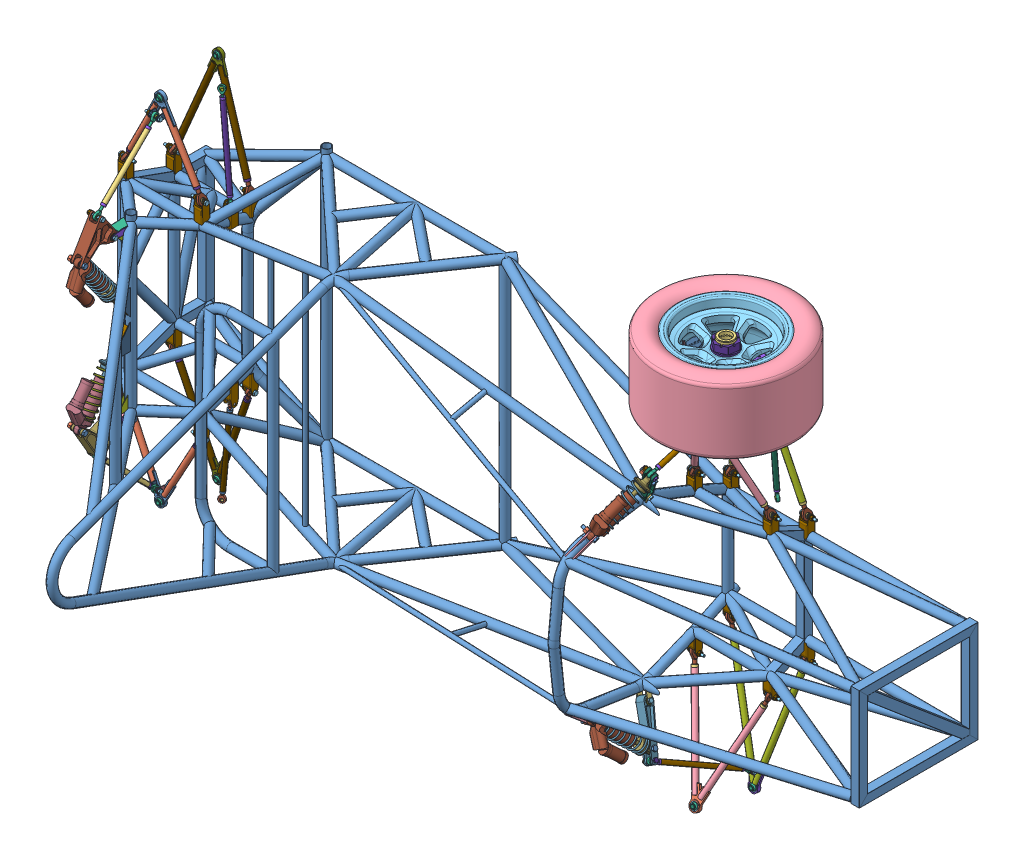
SolidWorks assembly AE-Rolling Chassis Assembly, configuration Default. Lengths in mm. (continued)
Components (placement in the parent): (continued)
- SP-A0200-AI-Rear Axle Assembly-1: SP-A0200-AI-Rear Axle Assembly [Default] at (222.4405 0 -72.1526) size (274.88 1137.82 484.64)
  - SP-AA-Rear Lower A-Arm^SP-A0200-AI-Rear Axle Assembly-1: SP-AA-Rear Lower A-Arm^SP-A0200-AI-Rear Axle Assembly [Default] at (0 -0.399 0.6588) x (1 0 0) z (0 0.002866 0.999996) size (222.76 290.57 36.42) (virtual)
    - SP-Lower Apex Rear-1: SP-Lower Apex Rear [Default] at (-792.4265 549.6462 121.5417) x (-0.932505 -0.360479 0.022123) z (0 -0.061256 -0.998122) size (54.94 63.8 9.53)
    - SP-10003-AB-Threaded Insert-1: SP-10003-AB-Threaded Insert [A-Arm] at (-890.6731 296.4508 137.0806) x (0.932505 -0.360479 0.022123) z (-0.361157 -0.930754 0.057121) size (15.88 15.88 15.88)
    - SP-10003-AB-Threaded Insert-2: SP-10003-AB-Threaded Insert [A-Arm] at (-694.18 296.4508 137.0806) x (0.932505 0.360479 -0.022123) z (0.361157 -0.930754 0.057121) size (15.88 15.88 15.88)
    - SP-Rear Lower A-Arm Tube-1: SP-Rear Lower A-Arm Tube [Default] at (-838.6322 430.5677 128.8497) x (-0.361157 -0.930754 0.057121) z (0 -0.061256 -0.998122) size (257.84 15.88 15.88)
    - SP-Rear Lower A-Arm Tube-2: SP-Rear Lower A-Arm Tube [Default] at (-746.2209 430.5677 128.8497) x (0.361157 -0.930754 0.057121) z (0 0.061256 0.998122) size (257.84 15.88 15.88)
    - FS-HIGH MISALIGN SPHERICAL BEARING, 0.375-0.906D (3072-6G)-1: FS-HIGH MISALIGN SPHERICAL BEARING, 0.375-0.906D (3072-6G) [Default] at (-792.4265 549.6462 121.5417) x (-0.932505 0.360479 -0.022123) z (-0.361157 -0.930754 0.057121) size (26.46 21.71 26.13)
      - Race^FS-HIGH MISALIGN SPHERICAL BEARING, 0.375-0.906D (3072-6G)-1: Race^FS-HIGH MISALIGN SPHERICAL BEARING, 0.375-0.906D (3072-6G) [Default] at origin size (23.01 8.76 23.01) (virtual)
      - Ball^FS-HIGH MISALIGN SPHERICAL BEARING, 0.375-0.906D (3072-6G)-1: Ball^FS-HIGH MISALIGN SPHERICAL BEARING, 0.375-0.906D (3072-6G) [Default] x (0.359576 -0.008176 0.93308) z (-0.932238 -0.046516 0.358844) size (19.84 20.65 19.84) (virtual)
  - SP-AA-Rear Upper A-Arm^SP-A0200-AI-Rear Axle Assembly-1: SP-AA-Rear Upper A-Arm^SP-A0200-AI-Rear Axle Assembly [Default] at (-38.1 -1.9308 1.9372) x (1 0 0) z (0 0.00685 0.999977) size (216 215.55 29.43) (virtual)
    - SP-Upper Apex Rear-1: SP-Upper Apex Rear [Default] at (-755.8405 523.8827 293.8505) x (0.884705 -0.465567 -0.023329) z (0 -0.050046 0.998747) size (76.45 83.12 9.53)
    - SP-10003-AB-Threaded Insert-1: SP-10003-AB-Threaded Insert [A-Arm] at (-849.4201 346.5014 284.9623) x (0.884705 -0.465567 -0.023329) z (-0.466151 -0.883596 -0.044276) size (15.88 15.88 15.88)
    - SP-10003-AB-Threaded Insert-2: SP-10003-AB-Threaded Insert [A-Arm] at (-662.261 346.5014 284.9623) x (0.884705 0.465567 0.023329) z (0.466151 -0.883596 -0.044276) size (15.88 15.88 15.88)
    - SP-Rear Upper A-Arm Tube-1: SP-Rear Upper A-Arm Tube [Default] at (-812.9905 415.5541 288.4224) x (0.466151 0.883596 0.044276) z (0.884705 -0.465567 -0.023329) size (186.28 15.88 15.88)
    - SP-Rear Upper A-Arm Tube-2: SP-Rear Upper A-Arm Tube [Default] at (-698.6905 415.5541 288.4224) x (-0.466151 0.883596 0.044276) z (0.884705 0.465567 0.023329) size (186.28 15.88 15.88)
    - FS-HIGH MISALIGN SPHERICAL BEARING, 0.375-0.906D (3072-6G)-1: FS-HIGH MISALIGN SPHERICAL BEARING, 0.375-0.906D (3072-6G) [Default] at (-755.8405 523.8827 293.8505) x (0.884705 -0.465567 -0.023329) z (-0.466151 -0.883596 -0.044276) size (26.46 21.71 26.13)
      - Race^FS-HIGH MISALIGN SPHERICAL BEARING, 0.375-0.906D (3072-6G)-1: Race^FS-HIGH MISALIGN SPHERICAL BEARING, 0.375-0.906D (3072-6G) [Default] at origin size (23.01 8.76 23.01) (virtual)
      - Ball^FS-HIGH MISALIGN SPHERICAL BEARING, 0.375-0.906D (3072-6G)-1: Ball^FS-HIGH MISALIGN SPHERICAL BEARING, 0.375-0.906D (3072-6G) [Default] x (0.359576 -0.008176 0.93308) z (-0.932238 -0.046516 0.358844) size (19.84 20.65 19.84) (virtual)
  - Assem8^SP-A0200-AI-Rear Axle Assembly-1: Assem8^SP-A0200-AI-Rear Axle Assembly [Default] at (-1592.9214 814.7933 712.2762) x (-0.999891 -0.01037 0.010464) z (0.012143 -0.982316 0.186836) size (17.98 166.51 230.13) (virtual)
    - Part2^Assem8_SP-A0200-AI-Rear Axle Assembly-1: Part2^Assem8_SP-A0200-AI-Rear Axle Assembly [Default] at origin size (15.39 113.92 157.78) (virtual)
    - SP-10003-AC-Threaded Insert-2: SP-10003-AC-Threaded Insert [AM-4 Rod End Thread] at (-799.064 427.6015 294.0449) x (-0.999891 -0.008342 0.012143) z (-0.014733 0.566176 -0.824153) size (12.7 12.7 15.88)
    - SP-10003-AC-Threaded Insert-3: SP-10003-AC-Threaded Insert [AM-4 Rod End Thread] at (-796.6527 334.9355 428.9338) x (-0.999891 -0.008342 0.012143) z (0.014733 -0.566176 0.824153) size (12.7 12.7 15.88)
    - FS-MALE ROD END UNF-3A, 0.25x28-0.25D (AM-4)-1: FS-MALE ROD END UNF-3A, 0.25x28-0.25D (AM-4) [Default] at (-796.0446 311.5665 462.9507) x (0 -0.824242 -0.566238) z (-0.014733 0.566176 -0.824153) size (19.32 14.06 49.44)
      - Body^FS-MALE ROD END UNF-3A, 0.25x28-0.25D (AM-4)-2: Body^FS-MALE ROD END UNF-3A, 0.25x28-0.25D (AM-4) [Default] at origin size (19.32 7.2 49.44) (virtual)
      - Ball^FS-MALE ROD END UNF-3A, 0.25x28-0.25D (AM-4)-2: Ball^FS-MALE ROD END UNF-3A, 0.25x28-0.25D (AM-4) [Default] x (0.09633 0.218783 0.971007) z (-0.984027 0.167661 0.059845) size (12.7 9.53 12.7) (virtual)
    - FS-MALE ROD END UNF-3A, 0.25x28-0.25D (AM-4)-2: FS-MALE ROD END UNF-3A, 0.25x28-0.25D (AM-4) [Default] at (-799.6721 450.9704 260.028) x (0 -0.824242 -0.566238) z (0.014733 -0.566176 0.824153) size (19.32 14.06 49.44)
      - Body^FS-MALE ROD END UNF-3A, 0.25x28-0.25D (AM-4)-2: Body^FS-MALE ROD END UNF-3A, 0.25x28-0.25D (AM-4) [Default] at origin size (19.32 7.2 49.44) (virtual)
      - Ball^FS-MALE ROD END UNF-3A, 0.25x28-0.25D (AM-4)-2: Ball^FS-MALE ROD END UNF-3A, 0.25x28-0.25D (AM-4) [Default] x (0.09633 0.218783 0.971007) z (-0.984027 0.167661 0.059845) size (12.7 9.53 12.7) (virtual)
  - SP-A0105-AC-Ohlin TTX25 MKII, 200mm-1: SP-A0105-AC-Ohlin TTX25 MKII, 200mm [Default] at (-793.9406 216.4917 537.8809) x (-1 0 0) z (0 0.803503 0.5953) size (48.39 85.02 197.6)
    - Shock Body^SP-A0105-AC-Ohlin TTX25 MKII, 200mm-1: Shock Body^SP-A0105-AC-Ohlin TTX25 MKII, 200mm [Default] at origin size (40.76 80 131.7) (virtual)
    - Head^SP-A0105-AC-Ohlin TTX25 MKII, 200mm-1: Head^SP-A0105-AC-Ohlin TTX25 MKII, 200mm [Default] at (0 0 -174.6) size (46 46 119) (virtual)
    - Ball^SP-A0105-AC-Ohlin TTX25 MKII, 200mm-1: Ball^SP-A0105-AC-Ohlin TTX25 MKII, 200mm [Default] at (0 0 -174.6) x (-0.011681 0.107343 0.994153) z (0.993776 0.111394 -0.000351) size (15 15 8) (virtual)
    - Ball^SP-A0105-AC-Ohlin TTX25 MKII, 200mm-2: Ball^SP-A0105-AC-Ohlin TTX25 MKII, 200mm [Default] x (0.079523 -0.862756 -0.499328) z (0.965926 -0.057074 0.252448) size (15 15 8) (virtual)
    - SP-#####-AB-Spring-1: SP-#####-AB-Spring [Default] at (0 0 -151.1) size (48.39 49.05 127.97)
  - FS-BALL BEARING, 0.25ID-0.75OD (60355K702)-1: FS-BALL BEARING, 0.25ID-0.75OD (60355K702) [Default] at (-784.8125 243.84 446.6415) x (0 -0.287121 0.957894) z (-1 0 0) size (19.05 19.05 7.14)
  - FS-BALL BEARING, 0.25ID-0.75OD (60355K702)-2: FS-BALL BEARING, 0.25ID-0.75OD (60355K702) [Default] at (-803.0688 243.84 446.6415) x (0 0.287121 -0.957894) z (1 0 0) size (19.05 19.05 7.14)
  - FS-CADMIUM PLATED C3 HEX, 0.25x28-1.65-0.469 (AN4-13A)-2: FS-CADMIUM PLATED C3 HEX, 0.25x28-1.65-0.469 (AN4-13A) [Default] at (-796.8362 310.0391 484.3789) x (-1 0 0) z (0 0.868755 0.495242) size (46.28 12.9 11.18)
  - FS-ZINC YELLOW CHROMATE C10.9 HX, M8x1.25-40-22 (95327A569)-1: FS-ZINC YELLOW CHROMATE C10.9 HX, M8x1.25-40-22 (95327A569) [Default] at (-795.4156 216.4917 537.8809) x (-1 0 0) z (0 -0.287121 0.957894) size (45.3 15.01 13)
  - FS-NYLOC FLHX C8, M8x1.25-11.1 (92461A400)-1: FS-NYLOC FLHX C8, M8x1.25-11.1 (92461A400) [Default] at (-820.9156 216.4917 537.8809) x (0 0.868058 -0.496463) z (-1 0 0) size (17.9 17.9 11.1)
  - FS-NYLOC G8 HX, 0.25x28-0.3125 (90630A145)-1: FS-NYLOC G8 HX, 0.25x28-0.3125 (90630A145) [Default] at (-809.8156 310.0391 484.3789) x (0 0.868058 -0.496463) z (0 0.496463 0.868058) size (11.11 7.94 12.83)
  - SP-C30066-AA-A-Arm Tab Box-1: SP-C30066-AA-A-Arm Tab Box [Default] at (-680.9758 289.7175 282.8202) x (-0.029021 0.999579 0) z (0 0 -1) size (60.32 25.4 25.4)
  - SP-C30066-AA-A-Arm Tab Box-2: SP-C30066-AA-A-Arm Tab Box [Default] at (-908.2405 289.7636 282.8202) x (0 1 0) z (0 0 -1) size (60.32 25.4 25.4)
  - SP-C30066-AA-A-Arm Tab Box-3: SP-C30066-AA-A-Arm Tab Box [Default] at (-678.1265 237.6164 139.5469) x (0 1 0) z (0 0 1) size (60.32 25.4 25.4)
  - SP-C30066-AA-A-Arm Tab Box-4: SP-C30066-AA-A-Arm Tab Box [Default] at (-906.7265 237.6164 139.5469) x (0 1 0) z (0 0 1) size (60.32 25.4 25.4)
  - SP-30063-AB- Front Pushrod Tab-1: SP-30063-AB- Front Pushrod Tab [Default] at (-782.0343 483.2134 293.6084) x (1 0 0) z (0 0.043203 -0.999066) size (1.59 15.88 23.81)
  - SP-30063-AB- Front Pushrod Tab-2: SP-30063-AB- Front Pushrod Tab [Default] at (-805.8468 483.2134 293.6084) x (-1 0 0) z (0 0.043203 -0.999066) size (1.59 15.88 23.81)
  - FS-NYLOC FLHX C8, M8x1.25-11.1 (92461A400)-2: FS-NYLOC FLHX C8, M8x1.25-11.1 (92461A400) [Default] at (-820.9156 243.84 446.6415) x (0 0 -1) z (-1 0 0) size (17.9 17.9 11.1)
  - FS-CADMIUM PLATED C3 HEX, 0.25x28-1.65-0.469 (AN4-13A)-3: FS-CADMIUM PLATED C3 HEX, 0.25x28-1.65-0.469 (AN4-13A) [Default] at (-796.8362 243.84 446.6415) x (-1 0 0) z (0 0.287121 -0.957894) size (46.28 12.9 11.18)
  - FS-CADMIUM PLATED C3 HEX, 0.25x28-1.65-0.469 (AN4-13A)-4: FS-CADMIUM PLATED C3 HEX, 0.25x28-1.65-0.469 (AN4-13A) [Default] at (-687.5506 306.9965 282.8202) x (-0.999579 -0.029021 0) z (0 0 -1) size (46.28 12.9 11.18)
  - FS-CADMIUM PLATED C3 HEX, 0.25x28-1.65-0.469 (AN4-13A)-5: FS-CADMIUM PLATED C3 HEX, 0.25x28-1.65-0.469 (AN4-13A) [Default] at (-902.1699 307.2261 282.8202) size (46.28 12.9 11.18)
  - FS-CADMIUM PLATED C3 HEX, 0.25x28-1.65-0.469 (AN4-13A)-6: FS-CADMIUM PLATED C3 HEX, 0.25x28-1.65-0.469 (AN4-13A) [Default] at (-912.7971 255.0789 139.5469) x (-1 0 0) z (0 0 -1) size (46.28 12.9 11.18)
  - FS-CADMIUM PLATED C3 HEX, 0.25x28-1.65-0.469 (AN4-13A)-7: FS-CADMIUM PLATED C3 HEX, 0.25x28-1.65-0.469 (AN4-13A) [Default] at (-684.1971 255.0789 139.5469) x (-1 0 0) z (0 0 -1) size (46.28 12.9 11.18)
  - FS-CADMIUM PLATED C3 HEX, 0.25x28-1.65-0.469 (AN4-13A)-8: FS-CADMIUM PLATED C3 HEX, 0.25x28-1.65-0.469 (AN4-13A) [Default] at (-799.2174 482.5275 309.4686) x (-1 0 0) z (0 -0.609051 0.793131) size (46.28 12.9 11.18)
  - FS-NYLOC G8 HX, 0.25x28-0.3125 (90630A145)-3: FS-NYLOC G8 HX, 0.25x28-0.3125 (90630A145) [Default] at (-807.4343 482.5275 309.4686) x (0 -0.043203 0.999066) z (0 -0.999066 -0.043203) size (11.11 7.94 12.83)
  - FS-NYLOC G8 HX, 0.25x28-0.3125 (90630A145)-4: FS-NYLOC G8 HX, 0.25x28-0.3125 (90630A145) [Default] at (-694.1772 306.8041 282.8202) x (-0.029021 0.999579 0) z (0 0 1) size (11.11 7.94 12.83)
  - FS-NYLOC G8 HX, 0.25x28-0.3125 (90630A145)-5: FS-NYLOC G8 HX, 0.25x28-0.3125 (90630A145) [Default] at (-895.5405 307.2261 282.8202) x (0 1 0) z (0 0 -1) size (11.11 7.94 12.83)
  - FS-NYLOC G8 HX, 0.25x28-0.3125 (90630A145)-6: FS-NYLOC G8 HX, 0.25x28-0.3125 (90630A145) [Default] at (-919.4265 255.0789 139.5469) x (0 1 0) z (0 0 1) size (11.11 7.94 12.83)
  - FS-NYLOC G8 HX, 0.25x28-0.3125 (90630A145)-7: FS-NYLOC G8 HX, 0.25x28-0.3125 (90630A145) [Default] at (-690.8265 255.0789 139.5469) x (0 -1 0) z (0 0 -1) size (11.11 7.94 12.83)
  - FS-ROD END RETAINING WASHER, 0.25-0.245 (NO PN)-5: FS-ROD END RETAINING WASHER, 0.25-0.245 (NO PN) [Default] at (-781.9073 482.5275 309.4686) x (0 1 0) z (-1 0 0) size (12.7 12.7 6.22)
  - FS-ROD END RETAINING WASHER, 0.25-0.245 (NO PN)-6: FS-ROD END RETAINING WASHER, 0.25-0.245 (NO PN) [Default] at (-805.9738 482.5275 309.4686) x (0 0.978954 0.204082) z (1 0 0) size (12.7 12.7 6.22)
  - SP-A0200-Rear Inner Rocker Gusset-1: SP-A0200-Rear Inner Rocker Gusset [Default] at (-793.9406 234.6955 425.4808) x (1 0 0) z (0 0.052336 0.99863) size (26.99 1.59 48.67)
  - SP-A0200-Rear Long Rocker Tab-1: SP-A0200-Rear Long Rocker Tab [Rear] at (-807.4344 243.84 446.6415) x (1 0 0) z (0 -0.00621 -0.999981) size (1.59 19.05 73.11)
  - SP-A0200-Rear Outer Rocker Gusset-1: SP-A0200-Rear Outer Rocker Gusset [Default] at (-793.9406 251.3902 418.9606) x (1 0 0) z (0 -0.039929 0.999203) size (26.99 1.59 43.52)
  - SP-A0200-Rear Rocker Gusset Support-1: SP-A0200-Rear Rocker Gusset Support [Default] at (-800.2906 228.5949 403.7833) x (0 0 1) z (0 1 0) size (38.05 1.59 40.09)
  - SP-A0200-Rear Short Rocker Tab-1: SP-A0200-Rear Short Rocker Tab [Rear] at (-780.4469 243.8408 446.6212) x (1 0 0) z (0 -0.00621 -0.999981) size (1.59 17.17 50.59)
  - SP-A0200-Rear Rocker Gusset Support-2: SP-A0200-Rear Rocker Gusset Support [Default] at (-789.8131 228.5949 403.7833) x (0 0 1) z (0 1 0) size (38.05 1.59 40.09)
  - SP-A0200-Rear Shock Gusset-1: SP-A0200-Rear Shock Gusset [Default] at (-793.9406 34.3591 413.4634) x (1 0 0) z (0 0.809017 0.587785) size (14.29 1.59 50.8)
  - SP-A0200-Rear Shock Tab-1: SP-A0200-Rear Shock Tab [Rear] at (-786.7969 76.2 433.9415) x (-1 0 0) z (0 -0.809017 -0.587785) size (1.59 45.95 88.76)
  - SP-A0200-Rear Shock Tab-2: SP-A0200-Rear Shock Tab [Front] at (-801.0844 76.2 433.9415) x (-1 0 0) z (0 -0.809017 -0.587785) size (1.59 45.95 88.76)
  - FS-MALE ROD END UNJF-3A, 0.375x24-0.25D (HXAM-4T)-4: FS-MALE ROD END UNJF-3A, 0.375x24-0.25D (HXAM-4T) [Simplified] at (-679.6405 307.2261 282.8202) x (0 0.043203 -0.999066) z (-0.466151 0.883879 0.038222) size (26.22 15.06 62.54)
    - Body^FS-MALE ROD END UNJF-3A, 0.375x24-0.25D (HXAM-4T)-1: Body^FS-MALE ROD END UNJF-3A, 0.375x24-0.25D (HXAM-4T) [no_threads] at origin size (26.22 9.62 62.54)
    - Ball^FS-MALE ROD END UNJF-3A, 0.375x24-0.25D (HXAM-4T)-1: Ball^FS-MALE ROD END UNJF-3A, 0.375x24-0.25D (HXAM-4T) [Default] at origin size (15.06 15.06 15.06)
  - FS-MALE ROD END UNJF-3A, 0.375x24-0.25D (HXAM-4T)-5: FS-MALE ROD END UNJF-3A, 0.375x24-0.25D (HXAM-4T) [Simplified] at (-908.2405 307.2261 282.8202) x (0 -0.043203 0.999066) z (0.466151 0.883879 0.038222) size (26.22 15.06 62.54)
    - Body^FS-MALE ROD END UNJF-3A, 0.375x24-0.25D (HXAM-4T)-1: Body^FS-MALE ROD END UNJF-3A, 0.375x24-0.25D (HXAM-4T) [no_threads] at origin size (26.22 9.62 62.54)
    - Ball^FS-MALE ROD END UNJF-3A, 0.375x24-0.25D (HXAM-4T)-1: Ball^FS-MALE ROD END UNJF-3A, 0.375x24-0.25D (HXAM-4T) [Default] at origin size (15.06 15.06 15.06)
  - FS-MALE ROD END UNJF-3A, 0.375x24-0.25D (HXAM-4T)-6: FS-MALE ROD END UNJF-3A, 0.375x24-0.25D (HXAM-4T) [Simplified] at (-906.7265 255.0789 139.5469) x (0 0.064116 0.997942) z (0.361157 0.930586 -0.059789) size (26.22 15.06 62.54)
    - Body^FS-MALE ROD END UNJF-3A, 0.375x24-0.25D (HXAM-4T)-1: Body^FS-MALE ROD END UNJF-3A, 0.375x24-0.25D (HXAM-4T) [no_threads] at origin size (26.22 9.62 62.54)
    - Ball^FS-MALE ROD END UNJF-3A, 0.375x24-0.25D (HXAM-4T)-1: Ball^FS-MALE ROD END UNJF-3A, 0.375x24-0.25D (HXAM-4T) [Default] at origin size (15.06 15.06 15.06)
  - FS-MALE ROD END UNJF-3A, 0.375x24-0.25D (HXAM-4T)-7: FS-MALE ROD END UNJF-3A, 0.375x24-0.25D (HXAM-4T) [Simplified] at (-678.1265 255.0789 139.5469) x (0 -0.064116 -0.997942) z (-0.361157 0.930586 -0.059789) size (26.22 15.06 62.54)
    - Body^FS-MALE ROD END UNJF-3A, 0.375x24-0.25D (HXAM-4T)-1: Body^FS-MALE ROD END UNJF-3A, 0.375x24-0.25D (HXAM-4T) [no_threads] at origin size (26.22 9.62 62.54)
    - Ball^FS-MALE ROD END UNJF-3A, 0.375x24-0.25D (HXAM-4T)-1: Ball^FS-MALE ROD END UNJF-3A, 0.375x24-0.25D (HXAM-4T) [Default] at origin size (15.06 15.06 15.06)
  - SP-B0100-Rear Rocker-1: SP-B0100-Rear Rocker [Default] at (14.7593 458.8134 -310.4211) x (0.993764 -0.111506 -0.000215) z (-0.085107 -0.759728 0.644647) size (43.51 92.41 122.03)
  - MirrorSP-B0100-Rear Rocker-2: MirrorSP-B0100-Rear Rocker [Default] at (14.7593 -458.8134 -310.4211) x (0.993764 0.111506 -0.000215) z (0.085107 -0.759728 -0.644647) size (43.51 92.41 122.03)
  - FS-MALE ROD END UNJF-3A, 0.375x24-0.25D (HXAM-4T)-8: FS-MALE ROD END UNJF-3A, 0.375x24-0.25D (HXAM-4T) [Simplified] at (-906.7265 -255.0789 139.5469) x (0 -0.064116 0.997942) z (0.361157 -0.930586 -0.059789) size (26.22 15.06 62.54)
    - Body^FS-MALE ROD END UNJF-3A, 0.375x24-0.25D (HXAM-4T)-1: Body^FS-MALE ROD END UNJF-3A, 0.375x24-0.25D (HXAM-4T) [no_threads] at origin size (26.22 9.62 62.54)
    - Ball^FS-MALE ROD END UNJF-3A, 0.375x24-0.25D (HXAM-4T)-1: Ball^FS-MALE ROD END UNJF-3A, 0.375x24-0.25D (HXAM-4T) [Default] at origin size (15.06 15.06 15.06)
  - FS-MALE ROD END UNJF-3A, 0.375x24-0.25D (HXAM-4T)-9: FS-MALE ROD END UNJF-3A, 0.375x24-0.25D (HXAM-4T) [Simplified] at (-908.2405 -307.2261 282.8202) x (0 0.043203 0.999066) z (0.466151 -0.883879 0.038222) size (26.22 15.06 62.54)
    - Body^FS-MALE ROD END UNJF-3A, 0.375x24-0.25D (HXAM-4T)-1: Body^FS-MALE ROD END UNJF-3A, 0.375x24-0.25D (HXAM-4T) [no_threads] at origin size (26.22 9.62 62.54)
    - Ball^FS-MALE ROD END UNJF-3A, 0.375x24-0.25D (HXAM-4T)-1: Ball^FS-MALE ROD END UNJF-3A, 0.375x24-0.25D (HXAM-4T) [Default] at origin size (15.06 15.06 15.06)
  - SP-A0200-Rear Shock Tab-3: SP-A0200-Rear Shock Tab [Front] at (-801.0844 -76.2 433.9415) x (1 0 0) z (0 0.809017 -0.587785) size (1.59 45.95 88.76)
  - SP-A0200-Rear Shock Gusset-2: SP-A0200-Rear Shock Gusset [Default] at (-793.9406 -34.3591 413.4634) x (-1 0 0) z (0 -0.809017 0.587785) size (14.29 1.59 50.8)
  - FS-CADMIUM PLATED C3 HEX, 0.25x28-1.65-0.469 (AN4-13A)-9: FS-CADMIUM PLATED C3 HEX, 0.25x28-1.65-0.469 (AN4-13A) [Default] at (-912.7971 -255.0789 139.5469) x (-1 0 0) z (0 0 1) size (46.28 12.9 11.18)
  - FS-ROD END RETAINING WASHER, 0.25-0.245 (NO PN)-7: FS-ROD END RETAINING WASHER, 0.25-0.245 (NO PN) [Default] at (-781.9073 -482.5275 309.4686) x (0 1 0) z (-1 0 0) size (12.7 12.7 6.22)
  - FS-NYLOC G8 HX, 0.25x28-0.3125 (90630A145)-8: FS-NYLOC G8 HX, 0.25x28-0.3125 (90630A145) [Default] at (-895.5405 -307.2261 282.8202) x (0 -1 0) z (0 0 1) size (11.11 7.94 12.83)
  - FS-CADMIUM PLATED C3 HEX, 0.25x28-1.65-0.469 (AN4-13A)-10: FS-CADMIUM PLATED C3 HEX, 0.25x28-1.65-0.469 (AN4-13A) [Default] at (-684.1971 -255.0789 139.5469) x (-1 0 0) z (0 0 1) size (46.28 12.9 11.18)
  - FS-NYLOC G8 HX, 0.25x28-0.3125 (90630A145)-9: FS-NYLOC G8 HX, 0.25x28-0.3125 (90630A145) [Default] at (-807.4343 -482.5275 309.4686) x (0 0.043203 0.999066) z (0 -0.999066 0.043203) size (11.11 7.94 12.83)
  - FS-CADMIUM PLATED C3 HEX, 0.25x28-1.65-0.469 (AN4-13A)-11: FS-CADMIUM PLATED C3 HEX, 0.25x28-1.65-0.469 (AN4-13A) [Default] at (-902.1699 -307.2261 282.8202) x (1 0 0) z (0 0 -1) size (46.28 12.9 11.18)
  - FS-CADMIUM PLATED C3 HEX, 0.25x28-1.65-0.469 (AN4-13A)-12: FS-CADMIUM PLATED C3 HEX, 0.25x28-1.65-0.469 (AN4-13A) [Default] at (-687.5506 -306.9965 282.8202) x (-0.999579 0.029021 0) z (0 0 1) size (46.28 12.9 11.18)
  - SP-A0200-Rear Short Rocker Tab-2: SP-A0200-Rear Short Rocker Tab [Rear] at (-780.4469 -243.8408 446.6212) x (-1 0 0) z (0 0.00621 -0.999981) size (1.59 17.17 50.59)
  - SP-A0200-Rear Long Rocker Tab-2: SP-A0200-Rear Long Rocker Tab [Rear] at (-807.4344 -243.84 446.6415) x (-1 0 0) z (0 0.00621 -0.999981) size (1.59 19.05 73.11)
  - FS-ROD END RETAINING WASHER, 0.25-0.245 (NO PN)-8: FS-ROD END RETAINING WASHER, 0.25-0.245 (NO PN) [Default] at (-805.9738 -482.5275 309.4686) x (0 0.978954 -0.204082) z (1 0 0) size (12.7 12.7 6.22)
  - FS-NYLOC G8 HX, 0.25x28-0.3125 (90630A145)-10: FS-NYLOC G8 HX, 0.25x28-0.3125 (90630A145) [Default] at (-694.1772 -306.8041 282.8202) x (-0.029021 -0.999579 0) z (0 0 -1) size (11.11 7.94 12.83)
  - FS-CADMIUM PLATED C3 HEX, 0.25x28-1.65-0.469 (AN4-13A)-13: FS-CADMIUM PLATED C3 HEX, 0.25x28-1.65-0.469 (AN4-13A) [Default] at (-799.2174 -482.5275 309.4686) x (-1 0 0) z (0 -0.609051 -0.793131) size (46.28 12.9 11.18)
  - FS-NYLOC G8 HX, 0.25x28-0.3125 (90630A145)-11: FS-NYLOC G8 HX, 0.25x28-0.3125 (90630A145) [Default] at (-690.8265 -255.0789 139.5469) x (0 1 0) z (0 0 1) size (11.11 7.94 12.83)
  - SP-A0200-Rear Inner Rocker Gusset-2: SP-A0200-Rear Inner Rocker Gusset [Default] at (-793.9406 -236.2808 425.3978) x (1 0 0) z (0 -0.052336 0.99863) size (26.99 1.59 48.67)
  - SP-A0200-Rear Rocker Gusset Support-3: SP-A0200-Rear Rocker Gusset Support [Default] at (-798.7031 -228.5949 403.7833) x (0 0 1) z (0 -1 0) size (38.05 1.59 40.09)
  - SP-A0200-Rear Outer Rocker Gusset-2: SP-A0200-Rear Outer Rocker Gusset [Default] at (-793.9406 -252.9764 419.024) x (1 0 0) z (0 0.039929 0.999203) size (26.99 1.59 43.52)
  - FS-MALE ROD END UNJF-3A, 0.375x24-0.25D (HXAM-4T)-10: FS-MALE ROD END UNJF-3A, 0.375x24-0.25D (HXAM-4T) [Simplified] at (-678.1265 -255.0789 139.5469) x (0 0.064116 -0.997942) z (-0.361157 -0.930586 -0.059789) size (26.22 15.06 62.54)
    - Body^FS-MALE ROD END UNJF-3A, 0.375x24-0.25D (HXAM-4T)-1: Body^FS-MALE ROD END UNJF-3A, 0.375x24-0.25D (HXAM-4T) [no_threads] at origin size (26.22 9.62 62.54)
    - Ball^FS-MALE ROD END UNJF-3A, 0.375x24-0.25D (HXAM-4T)-1: Ball^FS-MALE ROD END UNJF-3A, 0.375x24-0.25D (HXAM-4T) [Default] at origin size (15.06 15.06 15.06)
  - SP-A0200-Rear Rocker Gusset Support-4: SP-A0200-Rear Rocker Gusset Support [Default] at (-788.2256 -228.5949 403.7833) x (0 0 1) z (0 -1 0) size (38.05 1.59 40.09)
  - FS-MALE ROD END UNJF-3A, 0.375x24-0.25D (HXAM-4T)-11: FS-MALE ROD END UNJF-3A, 0.375x24-0.25D (HXAM-4T) [Simplified] at (-679.6405 -307.2261 282.8202) x (0 -0.043203 -0.999066) z (-0.466151 -0.883879 0.038222) size (26.22 15.06 62.54)
    - Body^FS-MALE ROD END UNJF-3A, 0.375x24-0.25D (HXAM-4T)-1: Body^FS-MALE ROD END UNJF-3A, 0.375x24-0.25D (HXAM-4T) [no_threads] at origin size (26.22 9.62 62.54)
    - Ball^FS-MALE ROD END UNJF-3A, 0.375x24-0.25D (HXAM-4T)-1: Ball^FS-MALE ROD END UNJF-3A, 0.375x24-0.25D (HXAM-4T) [Default] at origin size (15.06 15.06 15.06)
  - SP-A0200-Rear Shock Tab-4: SP-A0200-Rear Shock Tab [Rear] at (-786.7969 -76.2 433.9415) x (1 0 0) z (0 0.809017 -0.587785) size (1.59 45.95 88.76)
  - FS-NYLOC G8 HX, 0.25x28-0.3125 (90630A145)-12: FS-NYLOC G8 HX, 0.25x28-0.3125 (90630A145) [Default] at (-919.4265 -255.0789 139.5469) x (0 -1 0) z (0 0 -1) size (11.11 7.94 12.83)
  - SP-C30066-AA-A-Arm Tab Box-5: SP-C30066-AA-A-Arm Tab Box [Default] at (-680.9758 -289.7175 282.8202) x (-0.029021 -0.999579 0) z (0 0 1) size (60.32 25.4 25.4)
  - FS-NYLOC FLHX C8, M8x1.25-11.1 (92461A400)-3: FS-NYLOC FLHX C8, M8x1.25-11.1 (92461A400) [Default] at (-820.9156 -216.4917 537.8809) x (0 -0.868058 -0.496463) z (-1 0 0) size (17.9 17.9 11.1)
  - FS-CADMIUM PLATED C3 HEX, 0.25x28-1.65-0.469 (AN4-13A)-14: FS-CADMIUM PLATED C3 HEX, 0.25x28-1.65-0.469 (AN4-13A) [Default] at (-796.8362 -243.84 446.6415) x (-1 0 0) z (0 0.287121 0.957894) size (46.28 12.9 11.18)
  - SP-30063-AB- Front Pushrod Tab-3: SP-30063-AB- Front Pushrod Tab [Default] at (-807.4343 -483.2134 293.6084) x (1 0 0) z (0 -0.043203 -0.999066) size (1.59 15.88 23.81)
  - FS-BALL BEARING, 0.25ID-0.75OD (60355K702)-3: FS-BALL BEARING, 0.25ID-0.75OD (60355K702) [Default] at (-784.8125 -243.84 446.6415) x (0 -0.287121 -0.957894) z (-1 0 0) size (19.05 19.05 7.14)
  - MirrorSP-30063-AB- Front Pushrod Tab-4: MirrorSP-30063-AB- Front Pushrod Tab [Default] at (-782.0343 -483.2134 293.6084) x (1 0 0) z (0 0.043203 0.999066) size (1.59 15.88 23.81)
  - FS-CADMIUM PLATED C3 HEX, 0.25x28-1.65-0.469 (AN4-13A)-15: FS-CADMIUM PLATED C3 HEX, 0.25x28-1.65-0.469 (AN4-13A) [Default] at (-796.8362 -310.0391 484.3789) x (-1 0 0) z (0 0.868755 -0.495242) size (46.28 12.9 11.18)
  - Assem8^SP-A0200-AI-Rear Axle Assembly-2: Assem8^SP-A0200-AI-Rear Axle Assembly [Default] at (5.0402 21.5964 81.3981) x (0.999891 -0.01037 -0.010464) z (-0.012143 -0.982316 -0.186836) size (17.98 166.51 230.13) (virtual)
    - Part2^Assem8_SP-A0200-AI-Rear Axle Assembly-1: Part2^Assem8_SP-A0200-AI-Rear Axle Assembly [Default] at origin size (15.39 113.92 157.78) (virtual)
    - SP-10003-AC-Threaded Insert-2: SP-10003-AC-Threaded Insert [AM-4 Rod End Thread] at (-799.064 427.6015 294.0449) x (-0.999891 -0.008342 0.012143) z (-0.014733 0.566176 -0.824153) size (12.7 12.7 15.88)
    - SP-10003-AC-Threaded Insert-3: SP-10003-AC-Threaded Insert [AM-4 Rod End Thread] at (-796.6527 334.9355 428.9338) x (-0.999891 -0.008342 0.012143) z (0.014733 -0.566176 0.824153) size (12.7 12.7 15.88)
    - FS-MALE ROD END UNF-3A, 0.25x28-0.25D (AM-4)-1: FS-MALE ROD END UNF-3A, 0.25x28-0.25D (AM-4) [Default] at (-796.0446 311.5665 462.9507) x (0 -0.824242 -0.566238) z (-0.014733 0.566176 -0.824153) size (19.32 14.06 49.44)
      - Body^FS-MALE ROD END UNF-3A, 0.25x28-0.25D (AM-4)-2: Body^FS-MALE ROD END UNF-3A, 0.25x28-0.25D (AM-4) [Default] at origin size (19.32 7.2 49.44) (virtual)
      - Ball^FS-MALE ROD END UNF-3A, 0.25x28-0.25D (AM-4)-2: Ball^FS-MALE ROD END UNF-3A, 0.25x28-0.25D (AM-4) [Default] x (0.09633 0.218783 0.971007) z (-0.984027 0.167661 0.059845) size (12.7 9.53 12.7) (virtual)
    - FS-MALE ROD END UNF-3A, 0.25x28-0.25D (AM-4)-2: FS-MALE ROD END UNF-3A, 0.25x28-0.25D (AM-4) [Default] at (-799.6721 450.9704 260.028) x (0 -0.824242 -0.566238) z (0.014733 -0.566176 0.824153) size (19.32 14.06 49.44)
      - Body^FS-MALE ROD END UNF-3A, 0.25x28-0.25D (AM-4)-2: Body^FS-MALE ROD END UNF-3A, 0.25x28-0.25D (AM-4) [Default] at origin size (19.32 7.2 49.44) (virtual)
      - Ball^FS-MALE ROD END UNF-3A, 0.25x28-0.25D (AM-4)-2: Ball^FS-MALE ROD END UNF-3A, 0.25x28-0.25D (AM-4) [Default] x (0.09633 0.218783 0.971007) z (-0.984027 0.167661 0.059845) size (12.7 9.53 12.7) (virtual)
  - FS-BALL BEARING, 0.25ID-0.75OD (60355K702)-4: FS-BALL BEARING, 0.25ID-0.75OD (60355K702) [Default] at (-803.0688 -243.84 446.6415) x (0 0.287121 0.957894) z (1 0 0) size (19.05 19.05 7.14)
  - SP-AA-Rear Lower A-Arm^SP-A0200-AI-Rear Axle Assembly-2: SP-AA-Rear Lower A-Arm^SP-A0200-AI-Rear Axle Assembly [Default] at (-1584.8531 0.399 0.6588) x (-1 0 0) z (0 -0.002866 0.999996) size (222.76 290.57 36.42) (virtual)
    - SP-Lower Apex Rear-1: SP-Lower Apex Rear [Default] at (-792.4265 549.6462 121.5417) x (-0.932505 -0.360479 0.022123) z (0 -0.061256 -0.998122) size (54.94 63.8 9.53)
    - SP-10003-AB-Threaded Insert-1: SP-10003-AB-Threaded Insert [A-Arm] at (-890.6731 296.4508 137.0806) x (0.932505 -0.360479 0.022123) z (-0.361157 -0.930754 0.057121) size (15.88 15.88 15.88)
    - SP-10003-AB-Threaded Insert-2: SP-10003-AB-Threaded Insert [A-Arm] at (-694.18 296.4508 137.0806) x (0.932505 0.360479 -0.022123) z (0.361157 -0.930754 0.057121) size (15.88 15.88 15.88)
    - SP-Rear Lower A-Arm Tube-1: SP-Rear Lower A-Arm Tube [Default] at (-838.6322 430.5677 128.8497) x (-0.361157 -0.930754 0.057121) z (0 -0.061256 -0.998122) size (257.84 15.88 15.88)
    - SP-Rear Lower A-Arm Tube-2: SP-Rear Lower A-Arm Tube [Default] at (-746.2209 430.5677 128.8497) x (0.361157 -0.930754 0.057121) z (0 0.061256 0.998122) size (257.84 15.88 15.88)
    - FS-HIGH MISALIGN SPHERICAL BEARING, 0.375-0.906D (3072-6G)-1: FS-HIGH MISALIGN SPHERICAL BEARING, 0.375-0.906D (3072-6G) [Default] at (-792.4265 549.6462 121.5417) x (-0.932505 0.360479 -0.022123) z (-0.361157 -0.930754 0.057121) size (26.46 21.71 26.13)
      - Race^FS-HIGH MISALIGN SPHERICAL BEARING, 0.375-0.906D (3072-6G)-1: Race^FS-HIGH MISALIGN SPHERICAL BEARING, 0.375-0.906D (3072-6G) [Default] at origin size (23.01 8.76 23.01) (virtual)
      - Ball^FS-HIGH MISALIGN SPHERICAL BEARING, 0.375-0.906D (3072-6G)-1: Ball^FS-HIGH MISALIGN SPHERICAL BEARING, 0.375-0.906D (3072-6G) [Default] x (0.359576 -0.008176 0.93308) z (-0.932238 -0.046516 0.358844) size (19.84 20.65 19.84) (virtual)
  - FS-ZINC YELLOW CHROMATE C10.9 HX, M8x1.25-40-22 (95327A569)-2: FS-ZINC YELLOW CHROMATE C10.9 HX, M8x1.25-40-22 (95327A569) [Default] at (-795.4156 -216.4917 537.8809) x (-1 0 0) z (0 -0.287121 -0.957894) size (45.3 15.01 13)
  - FS-NYLOC FLHX C8, M8x1.25-11.1 (92461A400)-4: FS-NYLOC FLHX C8, M8x1.25-11.1 (92461A400) [Default] at (-820.9156 -243.84 446.6415) x (0 0 1) z (-1 0 0) size (17.9 17.9 11.1)
  - SP-C30066-AA-A-Arm Tab Box-6: SP-C30066-AA-A-Arm Tab Box [Default] at (-906.7265 -237.6164 139.5469) x (0 -1 0) z (0 0 -1) size (60.32 25.4 25.4)
  - SP-C30066-AA-A-Arm Tab Box-7: SP-C30066-AA-A-Arm Tab Box [Default] at (-678.1265 -237.6164 139.5469) x (0 -1 0) z (0 0 -1) size (60.32 25.4 25.4)
  - SP-C30066-AA-A-Arm Tab Box-8: SP-C30066-AA-A-Arm Tab Box [Default] at (-908.2405 -289.7636 282.8202) x (0 -1 0) z (0 0 1) size (60.32 25.4 25.4)
  - FS-NYLOC G8 HX, 0.25x28-0.3125 (90630A145)-13: FS-NYLOC G8 HX, 0.25x28-0.3125 (90630A145) [Default] at (-809.8156 -310.0391 484.3789) x (0 -0.868058 -0.496463) z (0 0.496463 -0.868058) size (11.11 7.94 12.83)
  - MirrorSP-A0105-AC-Ohlin TTX25 MKII, 200mm-2: MirrorSP-A0105-AC-Ohlin TTX25 MKII, 200mm [Default] at (-793.9406 -216.4917 537.8809) x (-1 0 0) z (0 0.803503 -0.5953) size (48.39 85.02 197.6)
    - MirrorShock Body^MirrorSP-A0105-AC-Ohlin TTX25 MKII, 200mm-1: MirrorShock Body^MirrorSP-A0105-AC-Ohlin TTX25 MKII, 200mm [Default] at origin size (40.76 80 131.7) (virtual)
    - MirrorHead^MirrorSP-A0105-AC-Ohlin TTX25 MKII, 200mm-1: MirrorHead^MirrorSP-A0105-AC-Ohlin TTX25 MKII, 200mm [Default] at (0 0 174.6) size (46 46 119) (virtual)
    - MirrorBall^MirrorSP-A0105-AC-Ohlin TTX25 MKII, 200mm-1: MirrorBall^MirrorSP-A0105-AC-Ohlin TTX25 MKII, 200mm [Default] at (0 0 174.6) x (-0.011681 0.107343 -0.994153) z (-0.993776 -0.111394 -0.000351) size (15 15 8) (virtual)
    - MirrorBall^MirrorSP-A0105-AC-Ohlin TTX25 MKII, 200mm-2: MirrorBall^MirrorSP-A0105-AC-Ohlin TTX25 MKII, 200mm [Default] x (0.079523 -0.862756 0.499328) z (-0.965926 0.057074 0.252448) size (15 15 8) (virtual)
    - MirrorSP-#####-AB-Spring-1: MirrorSP-#####-AB-Spring [Default] at (0 0 151.1) size (48.39 49.05 127.97)
  - SP-AA-Rear Upper A-Arm^SP-A0200-AI-Rear Axle Assembly-2: SP-AA-Rear Upper A-Arm^SP-A0200-AI-Rear Axle Assembly [Default] at (-1549.7811 1.9308 1.9372) x (-1 0 0) z (0 -0.00685 0.999977) size (216 215.55 29.43) (virtual)
    - SP-Upper Apex Rear-1: SP-Upper Apex Rear [Default] at (-755.8405 523.8827 293.8505) x (0.884705 -0.465567 -0.023329) z (0 -0.050046 0.998747) size (76.45 83.12 9.53)
    - SP-10003-AB-Threaded Insert-1: SP-10003-AB-Threaded Insert [A-Arm] at (-849.4201 346.5014 284.9623) x (0.884705 -0.465567 -0.023329) z (-0.466151 -0.883596 -0.044276) size (15.88 15.88 15.88)
    - SP-10003-AB-Threaded Insert-2: SP-10003-AB-Threaded Insert [A-Arm] at (-662.261 346.5014 284.9623) x (0.884705 0.465567 0.023329) z (0.466151 -0.883596 -0.044276) size (15.88 15.88 15.88)
    - SP-Rear Upper A-Arm Tube-1: SP-Rear Upper A-Arm Tube [Default] at (-812.9905 415.5541 288.4224) x (0.466151 0.883596 0.044276) z (0.884705 -0.465567 -0.023329) size (186.28 15.88 15.88)
    - SP-Rear Upper A-Arm Tube-2: SP-Rear Upper A-Arm Tube [Default] at (-698.6905 415.5541 288.4224) x (-0.466151 0.883596 0.044276) z (0.884705 0.465567 0.023329) size (186.28 15.88 15.88)
    - FS-HIGH MISALIGN SPHERICAL BEARING, 0.375-0.906D (3072-6G)-1: FS-HIGH MISALIGN SPHERICAL BEARING, 0.375-0.906D (3072-6G) [Default] at (-755.8405 523.8827 293.8505) x (0.884705 -0.465567 -0.023329) z (-0.466151 -0.883596 -0.044276) size (26.46 21.71 26.13)
      - Race^FS-HIGH MISALIGN SPHERICAL BEARING, 0.375-0.906D (3072-6G)-1: Race^FS-HIGH MISALIGN SPHERICAL BEARING, 0.375-0.906D (3072-6G) [Default] at origin size (23.01 8.76 23.01) (virtual)
      - Ball^FS-HIGH MISALIGN SPHERICAL BEARING, 0.375-0.906D (3072-6G)-1: Ball^FS-HIGH MISALIGN SPHERICAL BEARING, 0.375-0.906D (3072-6G) [Default] x (0.359576 -0.008176 0.93308) z (-0.932238 -0.046516 0.358844) size (19.84 20.65 19.84) (virtual)
  - SP-C30066-AA-A-Arm Tab Box-9: SP-C30066-AA-A-Arm Tab Box [Default] at (-678.1265 238.29 199.3134) x (0 1 0) z (0 0 1) size (60.32 25.4 25.4)
  - SP-####-AA-Rear Tie Rod Assem-1: SP-####-AA-Rear Tie Rod Assem [Default] at (-835.9968 207.5391 206.417) x (0.990379 0.133536 -0.036297) z (0.030001 0.048859 0.998355) size (23.87 299.22 22.34)
    - SP-####-AA-Rear Tie Rod-1: SP-####-AA-Rear Tie Rod [Default] at origin size (12.7 228.88 12.7)
    - SP-10003-AC-Threaded Insert-1: SP-10003-AC-Threaded Insert [AM-4 Rod End Thread] at (163.0475 271.467 0) x (1 0 0) z (0 1 0) size (12.7 12.7 15.88)
    - SP-10003-AC-Threaded Insert-2: SP-10003-AC-Threaded Insert [AM-4 Rod End Thread] at (163.0475 61.6371 0) x (-0.837169 0 -0.546944) z (0 -1 0) size (12.7 12.7 15.88)
    - FS-MALE ROD END UNF-3A, 0.25x28-0.25D (AM-4)-1: FS-MALE ROD END UNF-3A, 0.25x28-0.25D (AM-4) [Default] at (163.0475 306.392 0) x (-0.864851 0 0.502029) z (0 -1 0) size (19.32 14.06 49.44)
      - Body^FS-MALE ROD END UNF-3A, 0.25x28-0.25D (AM-4)-2: Body^FS-MALE ROD END UNF-3A, 0.25x28-0.25D (AM-4) [Default] at origin size (19.32 7.2 49.44) (virtual)
      - Ball^FS-MALE ROD END UNF-3A, 0.25x28-0.25D (AM-4)-2: Ball^FS-MALE ROD END UNF-3A, 0.25x28-0.25D (AM-4) [Default] x (0.09633 0.218783 0.971007) z (-0.984027 0.167661 0.059845) size (12.7 9.53 12.7) (virtual)
    - FS-MALE ROD END UNF-3A, 0.25x28-0.25D (AM-4)-2: FS-MALE ROD END UNF-3A, 0.25x28-0.25D (AM-4) [Default] at (163.0475 26.7121 0) x (-0.837169 0 -0.546944) z (0 1 0) size (19.32 14.06 49.44)
      - Body^FS-MALE ROD END UNF-3A, 0.25x28-0.25D (AM-4)-2: Body^FS-MALE ROD END UNF-3A, 0.25x28-0.25D (AM-4) [Default] at origin size (19.32 7.2 49.44) (virtual)
      - Ball^FS-MALE ROD END UNF-3A, 0.25x28-0.25D (AM-4)-2: Ball^FS-MALE ROD END UNF-3A, 0.25x28-0.25D (AM-4) [Default] x (0.09633 0.218783 0.971007) z (-0.984027 0.167661 0.059845) size (12.7 9.53 12.7) (virtual)
  - SP-C30066-AA-A-Arm Tab Box-10: SP-C30066-AA-A-Arm Tab Box [Default] at (-678.1265 -238.29 199.3134) x (0 -1 0) z (0 0 -1) size (60.32 25.4 25.4)
  - MirrorSP-####-AA-Rear Tie Rod Assem-2: MirrorSP-####-AA-Rear Tie Rod Assem [Default] at (-835.9968 -207.5391 206.417) x (0.990379 -0.133536 -0.036297) z (-0.030001 0.048859 -0.998355) size (23.87 299.22 22.34)
    - MirrorSP-####-AA-Rear Tie Rod-1: MirrorSP-####-AA-Rear Tie Rod [Default] at origin size (12.7 228.88 12.7)
    - MirrorSP-10003-AC-Threaded Insert-1: MirrorSP-10003-AC-Threaded Insert [AM-4 Rod End Thread] at (163.0475 271.467 0) x (1 0 0) z (0 -1 0) size (12.7 12.7 15.88)
    - MirrorSP-10003-AC-Threaded Insert-2: MirrorSP-10003-AC-Threaded Insert [AM-4 Rod End Thread] at (163.0475 61.6371 0) x (-0.837169 0 0.546944) z (0 1 0) size (12.7 12.7 15.88)
    - MirrorFS-MALE ROD END UNF-3A, 0.25x28-0.25D (AM-4)-1: MirrorFS-MALE ROD END UNF-3A, 0.25x28-0.25D (AM-4) [Default] at (163.0475 306.392 0) x (-0.864851 0 -0.502029) z (0 1 0) size (19.32 14.06 49.44)
      - MirrorBody^FS-MALE ROD END UNF-3A, 0.25x28-0-2: MirrorBody^FS-MALE ROD END UNF-3A, 0.25x28-0 [Default] at origin size (19.32 7.2 49.44)
      - MirrorBall^FS-MALE ROD END UNF-3A, 0.25x28-0-2: MirrorBall^FS-MALE ROD END UNF-3A, 0.25x28-0 [Default] x (0.09633 0.218783 -0.971007) z (0.984027 -0.167661 0.059845) size (12.7 9.53 12.7)
    - MirrorFS-MALE ROD END UNF-3A, 0.25x28-0.25D (AM-4)-2: MirrorFS-MALE ROD END UNF-3A, 0.25x28-0.25D (AM-4) [Default] at (163.0475 26.7121 0) x (-0.837169 0 0.546944) z (0 -1 0) size (19.32 14.06 49.44)
      - MirrorBody^FS-MALE ROD END UNF-3A, 0.25x28-0-2: MirrorBody^FS-MALE ROD END UNF-3A, 0.25x28-0 [Default] at origin size (19.32 7.2 49.44)
      - MirrorBall^FS-MALE ROD END UNF-3A, 0.25x28-0-2: MirrorBall^FS-MALE ROD END UNF-3A, 0.25x28-0 [Default] x (0.09633 0.218783 -0.971007) z (0.984027 -0.167661 0.059845) size (12.7 9.53 12.7)
